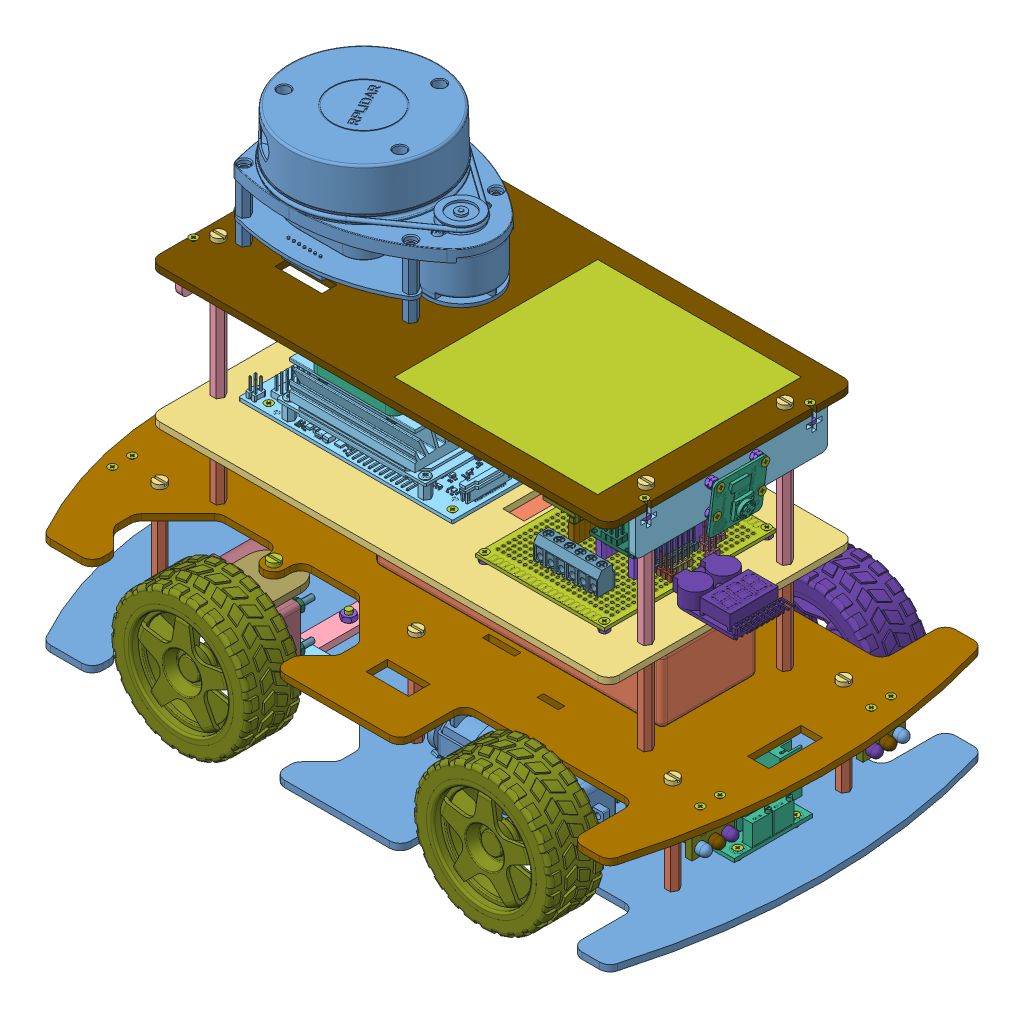
SolidWorks assembly Nigel - Motion Analysis, configuration Default. Lengths in mm. (continued)
Mates (geometry in assembly coordinates): (continued)
- Parallel7: parallel: plane of Platform 2-1 through (-150 43 0) normal (0 -1 0); plane of 5mm White LED-1 through (-135 31.99 33.75) normal (0 1 0)
- Concentric78: concentric: cylinder of LED Mount-2 through (-136 31.75 -33.75) axis (-1 0 0) radius 2.5; cylinder of 5mm White LED-2 through (-136 31.75 -33.75) axis (1 0 0) radius 2.5
- Coincident92: coincident: plane of LED Mount-2 through (-136 35.5 -40) normal (1 0 0); plane of 5mm White LED-2 through (-136 31.75 -33.75) normal (-1 0 0)
- Parallel8: parallel: plane of Platform 2-1 through (-150 43 0) normal (0 -1 0); plane of 5mm White LED-2 through (-135 31.99 -33.75) normal (0 1 0)
- Concentric79: concentric: cylinder of LED Mount-1 through (-136 31.75 40) axis (-1 0 0) radius 2.5; cylinder of 5mm White LED-3 through (-136 31.75 40) axis (1 0 0) radius 2.5
- Coincident94: coincident: plane of LED Mount-1 through (-136 35.5 40) normal (1 0 0); plane of 5mm White LED-3 through (-136 31.75 40) normal (-1 0 0)
- Parallel9: parallel: plane of Platform 2-1 through (-150 43 0) normal (0 -1 0); plane of 5mm White LED-3 through (-135 31.99 40) normal (0 1 0)
- Concentric80: concentric: cylinder of LED Mount-2 through (-136 31.75 -40) axis (-1 0 0) radius 2.5; cylinder of 5mm White LED-4 through (-136 31.75 -40) axis (1 0 0) radius 2.5
- Coincident96: coincident: plane of LED Mount-2 through (-136 35.5 -40) normal (1 0 0); plane of 5mm White LED-4 through (-136 31.75 -40) normal (-1 0 0)
- Parallel10: parallel: plane of Platform 2-1 through (-150 43 0) normal (0 -1 0); plane of 5mm White LED-4 through (-135 31.99 -40) normal (0 1 0)
- Concentric81: concentric: cylinder of LED Mount-3 through (139 31.75 33.75) axis (-1 0 0) radius 2.5; cylinder of 5mm White LED-5 through (136 31.75 33.75) axis (-1 0 0) radius 2.5
- Coincident99: coincident: plane of LED Mount-3 through (136 35.5 40) normal (-1 0 0); plane of 5mm White LED-5 through (136 31.75 33.75) normal (1 0 0)
- Parallel11: parallel: plane of Platform 2-1 through (-150 43 0) normal (0 -1 0); plane of 5mm White LED-5 through (135 31.99 33.75) normal (0 1 0)
- Concentric82: concentric: cylinder of LED Mount-4 through (139 31.75 -33.75) axis (-1 0 0) radius 2.5; cylinder of 5mm White LED-6 through (136 31.75 -33.75) axis (-1 0 0) radius 2.5
- Coincident100: coincident: plane of LED Mount-4 through (136 35.5 -40) normal (-1 0 0); plane of 5mm White LED-6 through (136 31.75 -33.75) normal (1 0 0)
- Parallel12: parallel: plane of Platform 2-1 through (-150 43 0) normal (0 -1 0); plane of 5mm White LED-6 through (135 31.99 -33.75) normal (0 1 0)
- Concentric83: concentric: cylinder of LED Mount-3 through (139 31.75 40) axis (-1 0 0) radius 2.5; cylinder of 5mm Red LED-1 through (136 31.75 40) axis (-1 0 0) radius 2.5
- Coincident103: coincident: plane of LED Mount-3 through (136 35.5 40) normal (-1 0 0); plane of 5mm Red LED-1 through (136 31.75 40) normal (1 0 0)
- Parallel13: parallel: plane of Platform 2-1 through (-150 43 0) normal (0 -1 0); plane of 5mm Red LED-1 through (135 31.99 40) normal (0 1 0)
- Concentric84: concentric: cylinder of LED Mount-4 through (139 31.75 -40) axis (-1 0 0) radius 2.5; cylinder of 5mm Red LED-2 through (136 31.75 -40) axis (-1 0 0) radius 2.5
- Coincident104: coincident: plane of LED Mount-4 through (136 35.5 -40) normal (-1 0 0); plane of 5mm Red LED-2 through (136 31.75 -40) normal (1 0 0)
- Parallel14: parallel: plane of Platform 2-1 through (-150 43 0) normal (0 -1 0); plane of 5mm Red LED-2 through (135 31.99 -40) normal (0 1 0)
- Concentric85: concentric: cylinder of LED Mount-1 through (-136 31.75 46.25) axis (-1 0 0) radius 2.5; cylinder of 5mm Amber LED-1 through (-136 31.75 46.25) axis (1 0 0) radius 2.5
- Coincident107: coincident: plane of LED Mount-1 through (-136 35.5 40) normal (1 0 0); plane of 5mm Amber LED-1 through (-136 31.75 46.25) normal (-1 0 0)
- Parallel15: parallel: plane of Platform 2-1 through (-150 43 0) normal (0 -1 0); plane of 5mm Amber LED-1 through (-135 31.99 46.25) normal (0 1 0)
- Concentric86: concentric: cylinder of LED Mount-2 through (-136 31.75 -46.25) axis (-1 0 0) radius 2.5; cylinder of 5mm Amber LED-2 through (-136 31.75 -46.25) axis (1 0 0) radius 2.5
- Coincident108: coincident: plane of LED Mount-2 through (-136 35.5 -40) normal (1 0 0); plane of 5mm Amber LED-2 through (-136 31.75 -46.25) normal (-1 0 0)
- Parallel16: parallel: plane of Platform 2-1 through (-150 43 0) normal (0 -1 0); plane of 5mm Amber LED-2 through (-135 31.99 -46.25) normal (0 1 0)
- Concentric87: concentric: cylinder of LED Mount-3 through (139 31.75 46.25) axis (-1 0 0) radius 2.5; cylinder of 5mm Amber LED-3 through (136 31.75 46.25) axis (-1 0 0) radius 2.5
- Coincident110: coincident: plane of LED Mount-3 through (136 35.5 40) normal (-1 0 0); plane of 5mm Amber LED-3 through (136 31.75 46.25) normal (1 0 0)
- Parallel17: parallel: plane of Platform 2-1 through (-150 43 0) normal (0 -1 0); plane of 5mm Amber LED-3 through (135 31.99 46.25) normal (0 1 0)
- Concentric88: concentric: cylinder of LED Mount-4 through (139 31.75 -46.25) axis (-1 0 0) radius 2.5; cylinder of 5mm Amber LED-4 through (136 31.75 -46.25) axis (-1 0 0) radius 2.5
- Coincident112: coincident: plane of LED Mount-4 through (136 35.5 -40) normal (-1 0 0); plane of 5mm Amber LED-4 through (136 31.75 -46.25) normal (1 0 0)
- Parallel18: parallel: plane of Platform 2-1 through (-150 43 0) normal (0 -1 0); plane of 5mm Amber LED-4 through (135 31.99 -46.25) normal (0 1 0)
- Concentric90: concentric: cylinder of Platform 1-1 through (-120 3 40) axis (0 -1 0) radius 1.6; cylinder of M3x40 F-F Standoff-1 through (-120 -1.2426 40) axis (0 1 0) radius 1.5
- Coincident115: coincident: plane of Platform 1-1 through (-150 3 0) normal (0 1 0); plane of M3x40 F-F Standoff-1 through (-120 3 40) normal (0 -1 0)
- Concentric91: concentric: cylinder of Platform 1-1 through (-120 3 -40) axis (0 -1 0) radius 1.6; cylinder of M3x40 F-F Standoff-2 through (-120 -1.2426 -40) axis (0 1 0) radius 1.5
- Coincident116: coincident: plane of Platform 1-1 through (-150 3 0) normal (0 1 0); plane of M3x40 F-F Standoff-2 through (-120 3 -40) normal (0 -1 0)
- Concentric92: concentric: cylinder of Platform 1-1 through (0 3 40) axis (0 -1 0) radius 1.6; cylinder of M3x40 F-F Standoff-3 through (0 -1.2426 40) axis (0 1 0) radius 1.5
- Coincident117: coincident: plane of Platform 1-1 through (-150 3 0) normal (0 1 0); plane of M3x40 F-F Standoff-3 through (0 3 40) normal (0 -1 0)
- Concentric93: concentric: cylinder of Platform 1-1 through (0 3 -40) axis (0 -1 0) radius 1.6; cylinder of M3x40 F-F Standoff-4 through (0 -1.2426 -40) axis (0 1 0) radius 1.5
- Coincident118: coincident: plane of Platform 1-1 through (-150 3 0) normal (0 1 0); plane of M3x40 F-F Standoff-4 through (0 3 -40) normal (0 -1 0)
- Concentric94: concentric: cylinder of Platform 1-1 through (120 3 40) axis (0 -1 0) radius 1.6; cylinder of M3x40 F-F Standoff-5 through (120 -1.2426 40) axis (0 1 0) radius 1.5
- Coincident119: coincident: plane of Platform 1-1 through (-150 3 0) normal (0 1 0); plane of M3x40 F-F Standoff-5 through (120 3 40) normal (0 -1 0)
- Concentric95: concentric: cylinder of Platform 1-1 through (120 3 -40) axis (0 -1 0) radius 1.6; cylinder of M3x40 F-F Standoff-6 through (120 -1.2426 -40) axis (0 1 0) radius 1.5
- Coincident120: coincident: plane of Platform 1-1 through (-150 3 0) normal (0 1 0); plane of M3x40 F-F Standoff-6 through (120 3 -40) normal (0 -1 0)
- Concentric106: concentric: cylinder of Platform 3-1 through (-80 89 29) axis (0 -1 0) radius 1.1; cylinder of Jetson Nano B01-1 through (-80 91.5 29) axis (0 1 0) radius 1.375
- Concentric107: concentric: cylinder of Platform 3-1 through (-80 89 -29) axis (0 -1 0) radius 1.1; cylinder of Jetson Nano B01-1 through (-80 91.5 -29) axis (0 1 0) radius 1.375
- Distance18: distance = 2.5 mm: plane of Jetson Nano B01-1 through (6 91.5 -29) normal (0 -1 0); plane of Platform 3-1 through (0 89 0) normal (0 1 0)
- Concentric110: concentric: cylinder of Platform 4-1 through (-92.5 152 28) axis (0 -1 0) radius 1.35; cylinder of RPLIDAR A1-1 through (-92.5 158 28) axis (0 -1 0) radius 1
- Concentric111: concentric: cylinder of Platform 4-1 through (-92.5 152 -28) axis (0 -1 0) radius 1.35; cylinder of RPLIDAR A1-1 through (-92.5 158 -28) axis (0 -1 0) radius 1
- Coincident132: coincident: plane of Platform 4-1 through (0 152 0) normal (0 1 0); plane of RPLIDAR A1-1 through (26.0533 152 -132.9176) normal (0 -1 0)
- Concentric112: concentric: cylinder of Platform 4-1 through (-71.5 152 -46.5) axis (0 -1 0) radius 1.1; cylinder of RPLIDAR Adapter-1 through (-71.5 150.2284 -46.5) axis (0 -1 0) radius 1
- Concentric113: concentric: cylinder of Platform 4-1 through (-57.5 152 -46.5) axis (0 -1 0) radius 1.1; cylinder of RPLIDAR Adapter-1 through (-57.5 150.2284 -46.5) axis (0 -1 0) radius 1
- Coincident133: coincident: plane of M2 Nut-45 through (-57.5 147.4 -46.5) normal (0 -1 0); plane of RPLIDAR Adapter-1 through (-64.5 147.4 -34) normal (0 1 0)
- Coincident142: coincident: plane of Platform 4-1 through (0 152 0) normal (0 1 0); plane of AprilTag-1 through (44.875 152 0) normal (0 -1 0)
- Distance19: distance = 9.875 mm: plane of AprilTag-1 through (-2.75 152.065 47.625) normal (0 0 1); plane of Platform 4-1 through (107.5 152 57.5) normal (0 0 1)
- Distance20: distance = 15 mm: plane of AprilTag-1 through (92.5 152.065 -47.625) normal (1 0 0); plane of Platform 4-1 through (107.5 152 39.8) normal (1 0 0)
- Concentric118: concentric: cylinder of Steering Link 2-2 through (-36.537 12 0) axis (0 -1 0) radius 1.6; cylinder of M3x25 Bolt-1 through (-36.537 34 0) axis (0 -1 0) radius 1.5
- Coincident143: coincident: plane of Steering Link 2-2 through (-36.537 9 -37.0517) normal (0 -1 0); plane of M3x25 Bolt-1 through (-36.537 9 0) normal (0 1 0)
- Slot1: slot: cylinder of M3x25 Bolt-1 through (-36.537 34 0) axis (0 -1 0) radius 1.5; cylinder of Acrylic Servo Horn-1 through (-39.0359 25.75 0) axis (0 -1 0) radius 1.6; cylinder of Acrylic Servo Horn-1 through (-34.0359 25.75 0) axis (0 -1 0) radius 1.6
- Parallel20: parallel: plane of Steering Link 1-2 through (-56.537 6 -45) normal (1 0 0); plane of Steering Link 2-2 through (-31.537 12 -37.0517) normal (1 0 0)
- Concentric119: concentric: cylinder of Platform 1-1 through (123.8 3 13.4) axis (0 -1 0) radius 1.1; cylinder of Buck Converter-2 through (123.8 7.15 13.4) axis (0 -1 0) radius 1.5
- Concentric120: concentric: cylinder of Platform 1-1 through (123.8 3 -13.4) axis (0 -1 0) radius 1.1; cylinder of Buck Converter-2 through (123.8 7.15 -13.4) axis (0 -1 0) radius 1.5
- Distance21: distance = 2.5 mm: plane of Buck Converter-2 through (94.4 5.5 0) normal (0 -1 0); plane of Platform 1-1 through (-150 3 0) normal (0 1 0)
- Coincident144: coincident: plane of Platform 4-1 through (0 149 0) normal (0 -1 0); plane of Front Camera Mount-1 through (-104.5 149 37.6) normal (0 1 0)
- Coincident145: coincident: plane of Platform 4-1 through (-107.5 152 -37.6) normal (-1 0 0); plane of Front Camera Mount-1 through (-107.5 140.25 0) normal (-1 0 0)
- Coincident146: coincident: plane of Platform 4-1 through (-107.5 152 39.8) normal (0 0 -1); plane of Front Camera Mount-1 through (-104.5 146.5 39.8) normal (0 0 -1)
- Coincident147: coincident: plane of Platform 4-1 through (0 149 0) normal (0 -1 0); plane of Rear Camera Mount-1 through (107.5 149 37.6) normal (0 1 0)
- Coincident148: coincident: plane of Platform 4-1 through (107.5 152 -37.6) normal (1 0 0); plane of Rear Camera Mount-1 through (107.5 140.25 0) normal (1 0 0)
- Coincident149: coincident: plane of Platform 4-1 through (104.5 152 37.6) normal (0 0 1); plane of Rear Camera Mount-1 through (107.5 149 37.6) normal (0 0 1)
- Concentric125: concentric: cylinder of Platform 1-1 through (36 3 0) axis (0 -1 0) radius 6.1; cylinder of M12 Push Button-1 through (36 12.74 0) axis (0 -1 0) radius 5.65
- Coincident152: coincident: plane of Platform 1-1 through (-150 0 0) normal (0 -1 0); plane of M12 Push Button-1 through (43 0 0) normal (0 1 0)
- Concentric126: concentric: cylinder of M12 Push Button-1 through (36 12.74 0) axis (0 -1 0) radius 5.65; cylinder of M12 Push Button Nut-1 through (36 5.3 0) axis (0 -1 0) radius 5.7643
- Coincident153: coincident: plane of Platform 1-1 through (-150 3 0) normal (0 1 0); plane of M12 Push Button Nut-1 through (36 3 0) normal (0 -1 0)
- Concentric127: concentric: cylinder of M3x25 Bolt-1 through (-36.537 34 0) axis (0 -1 0) radius 1.5; cylinder of M3 Nut-1 through (-36.537 14.4 0) axis (0 -1 0) radius 1.5
- Coincident154: coincident: plane of Steering Link 2-2 through (-36.537 12 -37.0517) normal (0 1 0); plane of M3 Nut-1 through (-36.537 12 0) normal (0 -1 0)
- Concentric128: concentric: cylinder of Platform 1-1 through (-61.537 3 -10) axis (0 -1 0) radius 1.6; cylinder of M3x10 Bolt-1 through (-61.537 10 -10) axis (0 -1 0) radius 1.5
- Coincident155: coincident: plane of Platform 1-1 through (-150 0 0) normal (0 -1 0); plane of M3x10 Bolt-1 through (-61.537 0 -10) normal (0 1 0)
- Concentric129: concentric: cylinder of Platform 1-1 through (-61.537 3 10) axis (0 -1 0) radius 1.6; cylinder of M3x10 Bolt-2 through (-61.537 10 10) axis (0 -1 0) radius 1.5
- Coincident156: coincident: plane of Platform 1-1 through (-150 0 0) normal (0 -1 0); plane of M3x10 Bolt-2 through (-61.537 0 10) normal (0 1 0)
- Concentric130: concentric: cylinder of M3x10 Bolt-1 through (-61.537 10 -10) axis (0 -1 0) radius 1.5; cylinder of M3 Nut-2 through (-61.537 8.4 -10) axis (0 -1 0) radius 1.5
- Coincident157: coincident: plane of Steering Link 1-2 through (-61.537 6 -45) normal (0 1 0); plane of M3 Nut-2 through (-61.537 6 -10) normal (0 -1 0)
- Concentric131: concentric: cylinder of M3x10 Bolt-2 through (-61.537 10 10) axis (0 -1 0) radius 1.5; cylinder of M3 Nut-3 through (-61.537 8.4 10) axis (0 -1 0) radius 1.5
- Coincident158: coincident: plane of Steering Link 1-2 through (-61.537 6 -45) normal (0 1 0); plane of M3 Nut-3 through (-61.537 6 10) normal (0 -1 0)
- Concentric138: concentric: cylinder of Steering Knuckle 1-1 through (-36.537 9 37.0517) axis (0 -1 0) radius 1.75; cylinder of M3x10 Bolt-3 through (-36.537 15.8 37.0517) axis (0 -1 0) radius 1.5
- Distance24: distance = 0.2 mm: plane of M3x10 Bolt-3 through (-36.537 5.8 37.0517) normal (0 1 0); plane of Steering Knuckle 1-1 through (-36.537 6 37.0517) normal (0 -1 0)
- Concentric141: concentric: cylinder of Steering Knuckle 1-2 through (-36.537 6 -37.0517) axis (0 1 0) radius 1.75; cylinder of M3x10 Bolt-4 through (-36.537 15.8 -37.0517) axis (0 -1 0) radius 1.5
- Distance27: distance = 0.2 mm: plane of Steering Knuckle 1-2 through (-36.537 6 -37.0517) normal (0 -1 0); plane of M3x10 Bolt-4 through (-36.537 5.8 -37.0517) normal (0 1 0)
- Concentric147: concentric: cylinder of M3 Nut-6 through (-36.537 14.4 37.0517) axis (0 -1 0) radius 1.5; cylinder of M3x10 Bolt-3 through (-36.537 15.8 37.0517) axis (0 -1 0) radius 1.5
- Coincident175: coincident: plane of Steering Link 2-2 through (-36.537 12 -37.0517) normal (0 1 0); plane of M3 Nut-6 through (-36.537 12 37.0517) normal (0 -1 0)
- Concentric148: concentric: cylinder of M3 Nut-7 through (-36.537 14.4 -37.0517) axis (0 -1 0) radius 1.5; cylinder of M3x10 Bolt-4 through (-36.537 15.8 -37.0517) axis (0 -1 0) radius 1.5
- Coincident176: coincident: plane of Steering Link 2-2 through (-36.537 12 -37.0517) normal (0 1 0); plane of M3 Nut-7 through (-36.537 12 -37.0517) normal (0 -1 0)
- Concentric149: concentric: cylinder of Platform 2-1 through (-61.537 46 45) axis (0 -1 0) radius 1.75; cylinder of M3x10 Bolt-5 through (-61.537 36 45) axis (0 1 0) radius 1.5
- Coincident177: coincident: plane of Platform 2-1 through (-150 46 0) normal (0 1 0); plane of M3x10 Bolt-5 through (-61.537 46 45) normal (0 -1 0)
- Concentric150: concentric: cylinder of M3 Nut-8 through (-61.537 39.8 45) axis (0 -1 0) radius 1.5; cylinder of M3x10 Bolt-5 through (-61.537 36 45) axis (0 1 0) radius 1.5
- Distance28: distance = 0.2 mm: plane of Steering Knuckle 2-1 through (-51.537 40 62.5) normal (0 -1 0); plane of M3 Nut-8 through (-61.537 39.8 45) normal (0 1 0)
- Concentric151: concentric: cylinder of Platform 2-1 through (-61.537 46 -45) axis (0 -1 0) radius 1.75; cylinder of M3x10 Bolt-6 through (-61.537 36 -45) axis (0 1 0) radius 1.5
- Coincident179: coincident: plane of Platform 2-1 through (-150 46 0) normal (0 1 0); plane of M3x10 Bolt-6 through (-61.537 46 -45) normal (0 -1 0)
- Concentric153: concentric: cylinder of M3 Nut-9 through (-61.537 39.8 -45) axis (0 -1 0) radius 1.5; cylinder of M3x10 Bolt-6 through (-61.537 36 -45) axis (0 1 0) radius 1.5
- Distance30: distance = 0.2 mm: plane of M3 Nut-9 through (-61.537 39.8 -45) normal (0 1 0); plane of Steering Knuckle 2-2 through (-71.537 40 -62.5) normal (0 -1 0)
- Concentric154: concentric: cylinder of Steering Knuckle 1-1 through (-61.537 9 45) axis (0 -1 0) radius 1.75; cylinder of M3x14 Bolt-1 through (-61.537 -5 45) axis (0 1 0) radius 1.5
- Coincident182: coincident: plane of Steering Knuckle 1-1 through (-36.537 9 37.0517) normal (0 1 0); plane of M3x14 Bolt-1 through (-61.537 9 45) normal (0 -1 0)
- Concentric155: concentric: cylinder of M3 Nut-4 through (-61.537 -0.2 45) axis (0 -1 0) radius 1.5; cylinder of M3x14 Bolt-1 through (-61.537 -5 45) axis (0 1 0) radius 1.5
- Distance31: distance = 0.2 mm: plane of M3 Nut-4 through (-61.537 -0.2 45) normal (0 1 0); plane of Platform 1-1 through (-150 0 0) normal (0 -1 0)
- Concentric156: concentric: cylinder of Steering Knuckle 1-2 through (-61.537 6 -45) axis (0 1 0) radius 1.75; cylinder of M3x14 Bolt-2 through (-61.537 -5 -45) axis (0 1 0) radius 1.5
- Coincident184: coincident: plane of Steering Knuckle 1-2 through (-36.537 9 -37.0517) normal (0 1 0); plane of M3x14 Bolt-2 through (-61.537 9 -45) normal (0 -1 0)
- Concentric157: concentric: cylinder of M3 Nut-5 through (-61.537 -0.2 -45) axis (0 -1 0) radius 1.5; cylinder of M3x14 Bolt-2 through (-61.537 -5 -45) axis (0 1 0) radius 1.5
- Distance32: distance = 0.2 mm: plane of Platform 1-1 through (-150 0 0) normal (0 -1 0); plane of M3 Nut-5 through (-61.537 -0.2 -45) normal (0 1 0)
- Concentric158: concentric: cylinder of Platform 1-1 through (-120 3 40) axis (0 -1 0) radius 1.6; cylinder of M3x8 Bolt-1 through (-120 8 40) axis (0 -1 0) radius 1.5
- Coincident186: coincident: plane of Platform 1-1 through (-150 0 0) normal (0 -1 0); plane of M3x8 Bolt-1 through (-120 0 40) normal (0 1 0)
- Concentric159: concentric: cylinder of Platform 1-1 through (-120 3 -40) axis (0 -1 0) radius 1.6; cylinder of M3x8 Bolt-2 through (-120 8 -40) axis (0 -1 0) radius 1.5
- Coincident187: coincident: plane of Platform 1-1 through (-150 0 0) normal (0 -1 0); plane of M3x8 Bolt-2 through (-120 0 -40) normal (0 1 0)
- Concentric160: concentric: cylinder of Platform 1-1 through (0 3 40) axis (0 -1 0) radius 1.6; cylinder of M3x8 Bolt-3 through (0 8 40) axis (0 -1 0) radius 1.5
- Coincident188: coincident: plane of Platform 1-1 through (-150 0 0) normal (0 -1 0); plane of M3x8 Bolt-3 through (0 0 40) normal (0 1 0)
- Concentric161: concentric: cylinder of Platform 1-1 through (0 3 -40) axis (0 -1 0) radius 1.6; cylinder of M3x8 Bolt-4 through (0 8 -40) axis (0 -1 0) radius 1.5
- Coincident189: coincident: plane of Platform 1-1 through (-150 0 0) normal (0 -1 0); plane of M3x8 Bolt-4 through (0 0 -40) normal (0 1 0)
- Concentric162: concentric: cylinder of Platform 1-1 through (120 3 40) axis (0 -1 0) radius 1.6; cylinder of M3x8 Bolt-5 through (120 8 40) axis (0 -1 0) radius 1.5
- Coincident190: coincident: plane of Platform 1-1 through (-150 0 0) normal (0 -1 0); plane of M3x8 Bolt-5 through (120 0 40) normal (0 1 0)
- Concentric163: concentric: cylinder of Platform 1-1 through (120 3 -40) axis (0 -1 0) radius 1.6; cylinder of M3x8 Bolt-6 through (120 8 -40) axis (0 -1 0) radius 1.5
- Coincident191: coincident: plane of Platform 1-1 through (-150 0 0) normal (0 -1 0); plane of M3x8 Bolt-6 through (120 0 -40) normal (0 1 0)
- Concentric164: concentric: cylinder of Platform 2-1 through (-120 46 40) axis (0 -1 0) radius 1.6; cylinder of M3x8 Bolt-7 through (-120 38 40) axis (0 1 0) radius 1.5
- Coincident192: coincident: plane of Platform 2-1 through (-150 46 0) normal (0 1 0); plane of M3x8 Bolt-7 through (-120 46 40) normal (0 -1 0)
- Concentric165: concentric: cylinder of Platform 2-1 through (-120 46 -40) axis (0 -1 0) radius 1.6; cylinder of M3x8 Bolt-8 through (-120 38 -40) axis (0 1 0) radius 1.5
- Coincident193: coincident: plane of Platform 2-1 through (-150 46 0) normal (0 1 0); plane of M3x8 Bolt-8 through (-120 46 -40) normal (0 -1 0)
- Concentric166: concentric: cylinder of Platform 2-1 through (0 46 40) axis (0 -1 0) radius 1.6; cylinder of M3x8 Bolt-9 through (0 38 40) axis (0 1 0) radius 1.5
- Coincident194: coincident: plane of Platform 2-1 through (-150 46 0) normal (0 1 0); plane of M3x8 Bolt-9 through (0 46 40) normal (0 -1 0)
- Concentric167: concentric: cylinder of Platform 2-1 through (0 46 -40) axis (0 -1 0) radius 1.6; cylinder of M3x8 Bolt-10 through (0 38 -40) axis (0 1 0) radius 1.5
- Coincident195: coincident: plane of Platform 2-1 through (-150 46 0) normal (0 1 0); plane of M3x8 Bolt-10 through (0 46 -40) normal (0 -1 0)
- Concentric168: concentric: cylinder of Platform 2-1 through (120 46 40) axis (0 -1 0) radius 1.6; cylinder of M3x8 Bolt-11 through (120 38 40) axis (0 1 0) radius 1.5
- Coincident196: coincident: plane of Platform 2-1 through (-150 46 0) normal (0 1 0); plane of M3x8 Bolt-11 through (120 46 40) normal (0 -1 0)
- Concentric169: concentric: cylinder of Platform 2-1 through (120 46 -40) axis (0 -1 0) radius 1.6; cylinder of M3x8 Bolt-12 through (120 38 -40) axis (0 1 0) radius 1.5
- Coincident197: coincident: plane of Platform 2-1 through (-150 46 0) normal (0 1 0); plane of M3x8 Bolt-12 through (120 46 -40) normal (0 -1 0)
- Concentric179: concentric: cylinder of Platform 1-1 through (65 3 13.4) axis (0 -1 0) radius 1.1; cylinder of M2x10 Bolt-5 through (65 8.4323 13.4) axis (0 1 0) radius 1
- Coincident207: coincident: circle of Buck Converter-2; cone of M2x10 Bolt-5 through (65 7.56 13.4) axis (0 -1 0)
- Concentric180: concentric: cylinder of Platform 1-1 through (65 3 -13.4) axis (0 -1 0) radius 1.1; cylinder of M2x10 Bolt-6 through (65 8.4323 -13.4) axis (0 1 0) radius 1
- Coincident208: coincident: circle of Buck Converter-2; cone of M2x10 Bolt-6 through (65 7.56 -13.4) axis (0 -1 0)
- Concentric181: concentric: cylinder of Platform 1-1 through (123.8 3 13.4) axis (0 -1 0) radius 1.1; cylinder of M2x10 Bolt-7 through (123.8 8.4323 13.4) axis (0 1 0) radius 1
- Coincident209: coincident: circle of Buck Converter-2; cone of M2x10 Bolt-7 through (123.8 7.56 13.4) axis (0 -1 0)
- Concentric182: concentric: cylinder of Platform 1-1 through (123.8 3 -13.4) axis (0 -1 0) radius 1.1; cylinder of M2x10 Bolt-8 through (123.8 8.4323 -13.4) axis (0 1 0) radius 1
- Coincident210: coincident: circle of Buck Converter-2; cone of M2x10 Bolt-8 through (123.8 7.56 -13.4) axis (0 -1 0)
- Concentric183: concentric: cylinder of M2x10 Bolt-5 through (65 8.4323 13.4) axis (0 1 0) radius 1; cylinder of M2 Nut-5 through (65 0 13.4) axis (0 -1 0) radius 1
- Coincident211: coincident: plane of Platform 1-1 through (-150 0 0) normal (0 -1 0); plane of M2 Nut-5 through (65 0 13.4) normal (0 1 0)
- Concentric184: concentric: cylinder of M2x10 Bolt-6 through (65 8.4323 -13.4) axis (0 1 0) radius 1; cylinder of M2 Nut-6 through (65 0 -13.4) axis (0 -1 0) radius 1
- Coincident212: coincident: plane of Platform 1-1 through (-150 0 0) normal (0 -1 0); plane of M2 Nut-6 through (65 0 -13.4) normal (0 1 0)
- Concentric185: concentric: cylinder of M2x10 Bolt-7 through (123.8 8.4323 13.4) axis (0 1 0) radius 1; cylinder of M2 Nut-7 through (123.8 0 13.4) axis (0 -1 0) radius 1
- Coincident213: coincident: plane of Platform 1-1 through (-150 0 0) normal (0 -1 0); plane of M2 Nut-7 through (123.8 0 13.4) normal (0 1 0)
- Concentric186: concentric: cylinder of M2x10 Bolt-8 through (123.8 8.4323 -13.4) axis (0 1 0) radius 1; cylinder of M2 Nut-8 through (123.8 0 -13.4) axis (0 -1 0) radius 1
- Coincident214: coincident: plane of Platform 1-1 through (-150 0 0) normal (0 -1 0); plane of M2 Nut-8 through (123.8 0 -13.4) normal (0 1 0)
- Concentric203: concentric: cylinder of Front Motor Mount-2 through (-53.037 31.75 60.5) axis (0 0 -1) radius 1.6; cylinder of M2.5x25 Bolt-1 through (-53.037 31.75 35.5) axis (0 0 1) radius 1.25
- Coincident231: coincident: plane of Front Motor Mount-2 through (-61.537 23 60.5) normal (0 0 1); plane of M2.5x25 Bolt-1 through (-53.037 31.75 60.5) normal (0 0 -1)
- Concentric205: concentric: cylinder of Front Motor Mount-2 through (-53.037 14.25 60.5) axis (0 0 -1) radius 1.6; cylinder of M2.5x25 Bolt-2 through (-53.037 14.25 35.5) axis (0 0 1) radius 1.25
- Coincident232: coincident: plane of Front Motor Mount-2 through (-61.537 23 60.5) normal (0 0 1); plane of M2.5x25 Bolt-2 through (-53.037 14.25 60.5) normal (0 0 -1)
- Concentric207: concentric: cylinder of Front Motor Mount-1 through (-53.037 31.75 -57.5) axis (0 0 -1) radius 1.6; cylinder of M2.5x25 Bolt-3 through (-53.037 31.75 -35.5) axis (0 0 -1) radius 1.25
- Coincident234: coincident: plane of Front Motor Mount-1 through (-61.537 23 -60.5) normal (0 0 -1); plane of M2.5x25 Bolt-3 through (-53.037 31.75 -60.5) normal (0 0 1)
- Concentric208: concentric: cylinder of Front Motor Mount-1 through (-53.037 14.25 -57.5) axis (0 0 -1) radius 1.6; cylinder of M2.5x25 Bolt-4 through (-53.037 14.25 -35.5) axis (0 0 -1) radius 1.25
- Coincident235: coincident: plane of Front Motor Mount-1 through (-61.537 23 -60.5) normal (0 0 -1); plane of M2.5x25 Bolt-4 through (-53.037 14.25 -60.5) normal (0 0 1)
- Concentric209: concentric: cylinder of M2.5x25 Bolt-1 through (-53.037 31.75 35.5) axis (0 0 1) radius 1.25; cylinder of M2.5 Nut-1 through (-53.037 31.75 43.5) axis (0 0 -1) radius 1.25
- Coincident236: coincident: plane of Front Wheel Hub-1 through (-92.537 34.25 43.5) normal (0 0 -1); plane of M2.5 Nut-1 through (-53.037 31.75 43.5) normal (0 0 1)
- Concentric210: concentric: cylinder of M2.5x25 Bolt-2 through (-53.037 14.25 35.5) axis (0 0 1) radius 1.25; cylinder of M2.5 Nut-2 through (-53.037 14.25 43.5) axis (0 0 -1) radius 1.25
- Coincident237: coincident: plane of Front Wheel Hub-1 through (-92.537 34.25 43.5) normal (0 0 -1); plane of M2.5 Nut-2 through (-53.037 14.25 43.5) normal (0 0 1)
- Concentric211: concentric: cylinder of M2.5x25 Bolt-3 through (-53.037 31.75 -35.5) axis (0 0 -1) radius 1.25; cylinder of M2.5 Nut-3 through (-53.037 31.75 -41.5) axis (0 0 -1) radius 1.25
- Coincident238: coincident: plane of Front Wheel Hub-2 through (-92.537 11.75 -43.5) normal (0 0 1); plane of M2.5 Nut-3 through (-53.037 31.75 -43.5) normal (0 0 -1)
- Concentric212: concentric: cylinder of M2.5x25 Bolt-4 through (-53.037 14.25 -35.5) axis (0 0 -1) radius 1.25; cylinder of M2.5 Nut-4 through (-53.037 14.25 -41.5) axis (0 0 -1) radius 1.25
- Coincident239: coincident: plane of Front Wheel Hub-2 through (-92.537 11.75 -43.5) normal (0 0 1); plane of M2.5 Nut-4 through (-53.037 14.25 -43.5) normal (0 0 -1)
- Concentric214: concentric: cylinder of Rear Motor Mount-2 through (59.4 31.75 37.9) axis (0 0 -1) radius 1.6; cylinder of M3x25 Bolt-2 through (59.4 31.75 31.5) axis (0 0 1) radius 1.5
- Coincident240: coincident: plane of Rear Motor-2 through (54.2 11.75 56.5) normal (0 0 1); plane of M3x25 Bolt-2 through (59.4 31.75 56.5) normal (0 0 -1)
- Concentric215: concentric: cylinder of Rear Motor Mount-2 through (59.4 14.25 37.9) axis (0 0 -1) radius 1.6; cylinder of M3x25 Bolt-3 through (59.4 14.25 31.5) axis (0 0 1) radius 1.5
- Coincident241: coincident: plane of Rear Motor-2 through (54.2 11.75 56.5) normal (0 0 1); plane of M3x25 Bolt-3 through (59.4 14.25 56.5) normal (0 0 -1)
- Concentric216: concentric: cylinder of Rear Motor Mount-1 through (59.4 31.75 -34.9) axis (0 0 -1) radius 1.6; cylinder of M3x25 Bolt-4 through (59.4 31.75 -31.5) axis (0 0 -1) radius 1.5
- Coincident242: coincident: plane of Rear Motor-1 through (54.2 34.25 -56.5) normal (0 0 -1); plane of M3x25 Bolt-4 through (59.4 31.75 -56.5) normal (0 0 1)
- Concentric217: concentric: cylinder of Rear Motor Mount-1 through (59.4 14.25 -34.9) axis (0 0 -1) radius 1.6; cylinder of M3x25 Bolt-5 through (59.4 14.25 -31.5) axis (0 0 -1) radius 1.5
- Coincident243: coincident: plane of Rear Motor-1 through (54.2 34.25 -56.5) normal (0 0 -1); plane of M3x25 Bolt-5 through (59.4 14.25 -56.5) normal (0 0 1)
- Concentric218: concentric: cylinder of M3x25 Bolt-2 through (59.4 31.75 31.5) axis (0 0 1) radius 1.5; cylinder of M3 Nut-10 through (59.4 31.75 34.9) axis (0 0 -1) radius 1.5
- Coincident244: coincident: plane of Rear Motor Mount-2 through (59.4 23 34.9) normal (0 0 -1); plane of M3 Nut-10 through (59.4 31.75 34.9) normal (0 0 1)
- Concentric219: concentric: cylinder of M3x25 Bolt-3 through (59.4 14.25 31.5) axis (0 0 1) radius 1.5; cylinder of M3 Nut-11 through (59.4 14.25 34.9) axis (0 0 -1) radius 1.5
- Coincident245: coincident: plane of Rear Motor Mount-2 through (59.4 23 34.9) normal (0 0 -1); plane of M3 Nut-11 through (59.4 14.25 34.9) normal (0 0 1)
- Concentric220: concentric: cylinder of M3x25 Bolt-4 through (59.4 31.75 -31.5) axis (0 0 -1) radius 1.5; cylinder of M3 Nut-12 through (59.4 31.75 -32.5) axis (0 0 -1) radius 1.5
- Coincident246: coincident: plane of Rear Motor Mount-1 through (59.4 23 -34.9) normal (0 0 1); plane of M3 Nut-12 through (59.4 31.75 -34.9) normal (0 0 -1)
- Concentric221: concentric: cylinder of M3x25 Bolt-5 through (59.4 14.25 -31.5) axis (0 0 -1) radius 1.5; cylinder of M3 Nut-13 through (59.4 14.25 -32.5) axis (0 0 -1) radius 1.5
- Coincident247: coincident: plane of Rear Motor Mount-1 through (59.4 23 -34.9) normal (0 0 1); plane of M3 Nut-13 through (59.4 14.25 -34.9) normal (0 0 -1)
- Concentric222: concentric: cylinder of Platform 2-1 through (-100 46 32.5) axis (0 -1 0) radius 1.6; cylinder of M3x8 Bolt-13 through (-100 51 32.5) axis (0 -1 0) radius 1.5
- Coincident248: coincident: plane of Platform 2-1 through (-150 43 0) normal (0 -1 0); plane of M3x8 Bolt-13 through (-100 43 32.5) normal (0 1 0)
- Concentric223: concentric: cylinder of Platform 2-1 through (-100 46 -32.5) axis (0 -1 0) radius 1.6; cylinder of M3x8 Bolt-14 through (-100 51 -32.5) axis (0 -1 0) radius 1.5
- Coincident249: coincident: plane of Platform 2-1 through (-150 43 0) normal (0 -1 0); plane of M3x8 Bolt-14 through (-100 43 -32.5) normal (0 1 0)
- Concentric224: concentric: cylinder of Platform 2-1 through (100 46 32.5) axis (0 -1 0) radius 1.6; cylinder of M3x8 Bolt-15 through (100 51 32.5) axis (0 -1 0) radius 1.5
- Coincident250: coincident: plane of Platform 2-1 through (-150 43 0) normal (0 -1 0); plane of M3x8 Bolt-15 through (100 43 32.5) normal (0 1 0)
- Concentric225: concentric: cylinder of Platform 2-1 through (100 46 -32.5) axis (0 -1 0) radius 1.6; cylinder of M3x8 Bolt-16 through (100 51 -32.5) axis (0 -1 0) radius 1.5
- Coincident251: coincident: plane of Platform 2-1 through (-150 43 0) normal (0 -1 0); plane of M3x8 Bolt-16 through (100 43 -32.5) normal (0 1 0)
- Concentric226: concentric: cylinder of Platform 2-1 through (-93.847 46 4.925) axis (0 -1 0) radius 2.1; cylinder of M4x10 Bolt-1 through (-93.847 36 4.925) axis (0 1 0) radius 2
- Coincident252: coincident: plane of Platform 2-1 through (-150 46 0) normal (0 1 0); plane of M4x10 Bolt-1 through (-93.847 46 4.925) normal (0 -1 0)
- Concentric227: concentric: cylinder of Platform 2-1 through (-93.847 46 -4.925) axis (0 -1 0) radius 2.1; cylinder of M4x10 Bolt-2 through (-93.847 36 -4.925) axis (0 1 0) radius 2
- Coincident253: coincident: plane of Platform 2-1 through (-150 46 0) normal (0 1 0); plane of M4x10 Bolt-2 through (-93.847 46 -4.925) normal (0 -1 0)
- Concentric228: concentric: cylinder of Platform 2-1 through (-43.327 46 4.925) axis (0 -1 0) radius 2.1; cylinder of M4x10 Bolt-3 through (-43.327 36 4.925) axis (0 1 0) radius 2
- Coincident254: coincident: plane of Platform 2-1 through (-150 46 0) normal (0 1 0); plane of M4x10 Bolt-3 through (-43.327 46 4.925) normal (0 -1 0)
- Concentric229: concentric: cylinder of Platform 2-1 through (-43.327 46 -4.925) axis (0 -1 0) radius 2.1; cylinder of M4x10 Bolt-4 through (-43.327 36 -4.925) axis (0 1 0) radius 2
- Coincident255: coincident: plane of Platform 2-1 through (-150 46 0) normal (0 1 0); plane of M4x10 Bolt-4 through (-43.327 46 -4.925) normal (0 -1 0)
- Concentric230: concentric: cylinder of M4x10 Bolt-1 through (-93.847 36 4.925) axis (0 1 0) radius 2; cylinder of M4 Nut-1 through (-93.847 40.6 4.925) axis (0 -1 0) radius 2
- Coincident256: coincident: plane of MG996R Servo Motor-1 through (-95.8964 40.6 6.525) normal (0 -1 0); plane of M4 Nut-1 through (-93.847 40.6 4.925) normal (0 1 0)
- Concentric231: concentric: cylinder of M4x10 Bolt-2 through (-93.847 36 -4.925) axis (0 1 0) radius 2; cylinder of M4 Nut-2 through (-93.847 40.6 -4.925) axis (0 -1 0) radius 2
- Coincident257: coincident: plane of MG996R Servo Motor-1 through (-95.8964 40.6 6.525) normal (0 -1 0); plane of M4 Nut-2 through (-93.847 40.6 -4.925) normal (0 1 0)
- Concentric232: concentric: cylinder of M4x10 Bolt-3 through (-43.327 36 4.925) axis (0 1 0) radius 2; cylinder of M4 Nut-3 through (-43.327 40.6 4.925) axis (0 -1 0) radius 2
- Coincident258: coincident: plane of MG996R Servo Motor-1 through (-95.8964 40.6 6.525) normal (0 -1 0); plane of M4 Nut-3 through (-43.327 40.6 4.925) normal (0 1 0)
- Concentric233: concentric: cylinder of M4x10 Bolt-4 through (-43.327 36 -4.925) axis (0 1 0) radius 2; cylinder of M4 Nut-4 through (-43.327 40.6 -4.925) axis (0 -1 0) radius 2
- Coincident259: coincident: plane of MG996R Servo Motor-1 through (-95.8964 40.6 6.525) normal (0 -1 0); plane of M4 Nut-4 through (-43.327 40.6 -4.925) normal (0 1 0)
- Concentric234: concentric: cylinder of MG996R Servo Horn-1 through (-59.0359 25.75 0) axis (0 1 0) radius 1.5; cylinder of M3x6 Bolt-1 through (-59.0359 31.75 0) axis (0 -1 0) radius 1.5
- Coincident260: coincident: plane of MG996R Servo Horn-1 through (-59.0359 25.75 0) normal (0 -1 0); plane of M3x6 Bolt-1 through (-59.0359 25.75 0) normal (0 1 0)
- Concentric235: concentric: cylinder of Acrylic Servo Horn-1 through (-66.0359 25.75 0) axis (0 -1 0) radius 1.6; cylinder of M3x6 Bolt-2 through (-66.0359 28.75 0) axis (0 -1 0) radius 1.5
- Coincident261: coincident: plane of Acrylic Servo Horn-1 through (-34.0359 22.75 0) normal (0 -1 0); plane of M3x6 Bolt-2 through (-66.0359 22.75 0) normal (0 1 0)
- Concentric236: concentric: cylinder of Acrylic Servo Horn-1 through (-59.0359 25.75 7) axis (0 -1 0) radius 1.6; cylinder of M3x6 Bolt-3 through (-59.0359 28.75 7) axis (0 -1 0) radius 1.5
- Coincident262: coincident: plane of Acrylic Servo Horn-1 through (-34.0359 22.75 0) normal (0 -1 0); plane of M3x6 Bolt-3 through (-59.0359 22.75 7) normal (0 1 0)
- Concentric237: concentric: cylinder of Acrylic Servo Horn-1 through (-52.0359 25.75 0) axis (0 -1 0) radius 1.6; cylinder of M3x6 Bolt-4 through (-52.0359 28.75 0) axis (0 -1 0) radius 1.5
- Coincident263: coincident: plane of Acrylic Servo Horn-1 through (-34.0359 22.75 0) normal (0 -1 0); plane of M3x6 Bolt-4 through (-52.0359 22.75 0) normal (0 1 0)
- Concentric238: concentric: cylinder of Acrylic Servo Horn-1 through (-59.0359 25.75 -7) axis (0 -1 0) radius 1.6; cylinder of M3x6 Bolt-5 through (-59.0359 28.75 -7) axis (0 -1 0) radius 1.5
- Coincident264: coincident: plane of Acrylic Servo Horn-1 through (-34.0359 22.75 0) normal (0 -1 0); plane of M3x6 Bolt-5 through (-59.0359 22.75 -7) normal (0 1 0)
- Concentric239: concentric: cylinder of M3x25 Bolt-1 through (-36.537 34 0) axis (0 -1 0) radius 1.5; cylinder of M3 Nut-14 through (-36.537 28.15 0) axis (0 -1 0) radius 1.5
- Coincident265: coincident: plane of Acrylic Servo Horn-1 through (-34.0359 25.75 0) normal (0 1 0); plane of M3 Nut-14 through (-36.537 25.75 0) normal (0 -1 0)
- Concentric240: concentric: cylinder of Platform 2-1 through (-137.5 46 44.6) axis (0 -1 0) radius 1.1; cylinder of M2x10 Bolt-9 through (-137.5 47.6723 44.6) axis (0 1 0) radius 1
- Coincident266: coincident: circle of Platform 2-1; cone of M2x10 Bolt-9 through (-137.5 46.8 44.6) axis (0 -1 0)
- Concentric241: concentric: cylinder of M2x10 Bolt-9 through (-137.5 47.6723 44.6) axis (0 1 0) radius 1; cylinder of M2 Nut-9 through (-137.5 40.5 44.6) axis (0 -1 0) radius 1
- Coincident267: coincident: plane of LED Mount-1 through (-136 40.5 40) normal (0 -1 0); plane of M2 Nut-9 through (-137.5 40.5 44.6) normal (0 1 0)
- Concentric242: concentric: cylinder of Platform 2-1 through (-137.5 46 35.4) axis (0 -1 0) radius 1.1; cylinder of M2x10 Bolt-10 through (-137.5 47.6723 35.4) axis (0 1 0) radius 1
- Coincident268: coincident: circle of Platform 2-1; cone of M2x10 Bolt-10 through (-137.5 46.8 35.4) axis (0 -1 0)
- Concentric243: concentric: cylinder of M2x10 Bolt-10 through (-137.5 47.6723 35.4) axis (0 1 0) radius 1; cylinder of M2 Nut-10 through (-137.5 40.5 35.4) axis (0 -1 0) radius 1
- Coincident269: coincident: plane of LED Mount-1 through (-136 40.5 40) normal (0 -1 0); plane of M2 Nut-10 through (-137.5 40.5 35.4) normal (0 1 0)
- Concentric244: concentric: cylinder of Platform 2-1 through (-137.5 46 -35.4) axis (0 -1 0) radius 1.1; cylinder of M2x10 Bolt-11 through (-137.5 47.6723 -35.4) axis (0 1 0) radius 1
- Coincident270: coincident: circle of Platform 2-1; cone of M2x10 Bolt-11 through (-137.5 46.8 -35.4) axis (0 -1 0)
- Concentric245: concentric: cylinder of M2x10 Bolt-11 through (-137.5 47.6723 -35.4) axis (0 1 0) radius 1; cylinder of M2 Nut-11 through (-137.5 40.5 -35.4) axis (0 -1 0) radius 1
- Coincident271: coincident: plane of LED Mount-2 through (-136 40.5 -40) normal (0 -1 0); plane of M2 Nut-11 through (-137.5 40.5 -35.4) normal (0 1 0)
- Concentric246: concentric: cylinder of Platform 2-1 through (-137.5 46 -44.6) axis (0 -1 0) radius 1.1; cylinder of M2x10 Bolt-12 through (-137.5 47.6723 -44.6) axis (0 1 0) radius 1
- Coincident272: coincident: circle of Platform 2-1; cone of M2x10 Bolt-12 through (-137.5 46.8 -44.6) axis (0 -1 0)
- Concentric247: concentric: cylinder of M2x10 Bolt-12 through (-137.5 47.6723 -44.6) axis (0 1 0) radius 1; cylinder of M2 Nut-12 through (-137.5 40.5 -44.6) axis (0 -1 0) radius 1
- Coincident273: coincident: plane of LED Mount-2 through (-136 40.5 -40) normal (0 -1 0); plane of M2 Nut-12 through (-137.5 40.5 -44.6) normal (0 1 0)
- Concentric248: concentric: cylinder of Platform 2-1 through (137.5 46 44.6) axis (0 -1 0) radius 1.1; cylinder of M2x10 Bolt-13 through (137.5 47.6723 44.6) axis (0 1 0) radius 1
- Coincident274: coincident: circle of Platform 2-1; cone of M2x10 Bolt-13 through (137.5 46.8 44.6) axis (0 -1 0)
- Concentric249: concentric: cylinder of M2x10 Bolt-13 through (137.5 47.6723 44.6) axis (0 1 0) radius 1; cylinder of M2 Nut-13 through (137.5 40.5 44.6) axis (0 -1 0) radius 1
- Coincident275: coincident: plane of LED Mount-3 through (139 40.5 40) normal (0 -1 0); plane of M2 Nut-13 through (137.5 40.5 44.6) normal (0 1 0)
- Concentric250: concentric: cylinder of Platform 2-1 through (137.5 46 35.4) axis (0 -1 0) radius 1.1; cylinder of M2x10 Bolt-14 through (137.5 47.6723 35.4) axis (0 1 0) radius 1
- Coincident276: coincident: circle of Platform 2-1; cone of M2x10 Bolt-14 through (137.5 46.8 35.4) axis (0 -1 0)
- Concentric251: concentric: cylinder of M2x10 Bolt-14 through (137.5 47.6723 35.4) axis (0 1 0) radius 1; cylinder of M2 Nut-14 through (137.5 40.5 35.4) axis (0 -1 0) radius 1
- Coincident277: coincident: plane of LED Mount-3 through (139 40.5 40) normal (0 -1 0); plane of M2 Nut-14 through (137.5 40.5 35.4) normal (0 1 0)
- Concentric252: concentric: cylinder of Platform 2-1 through (137.5 46 -35.4) axis (0 -1 0) radius 1.1; cylinder of M2x10 Bolt-15 through (137.5 47.6723 -35.4) axis (0 1 0) radius 1
- Coincident278: coincident: circle of Platform 2-1; cone of M2x10 Bolt-15 through (137.5 46.8 -35.4) axis (0 -1 0)
- Concentric253: concentric: cylinder of M2x10 Bolt-15 through (137.5 47.6723 -35.4) axis (0 1 0) radius 1; cylinder of M2 Nut-15 through (137.5 40.5 -35.4) axis (0 -1 0) radius 1
- Coincident279: coincident: plane of LED Mount-4 through (139 40.5 -40) normal (0 -1 0); plane of M2 Nut-15 through (137.5 40.5 -35.4) normal (0 1 0)
- Concentric254: concentric: cylinder of Platform 2-1 through (137.5 46 -44.6) axis (0 -1 0) radius 1.1; cylinder of M2x10 Bolt-16 through (137.5 47.6723 -44.6) axis (0 1 0) radius 1
